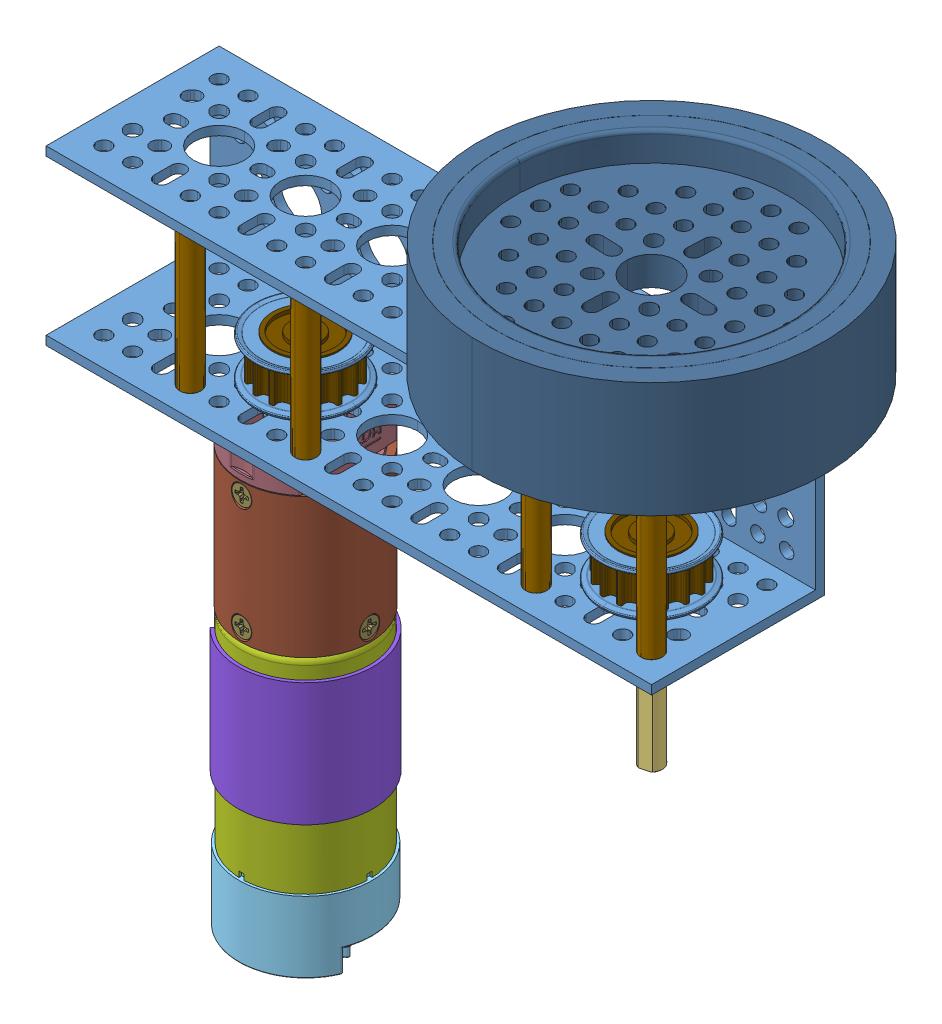
SolidWorks assembly motorisationDroite, configuration Défaut. Lengths in mm.
Overall size (193.77 212.25 99.53).
69 component instances, 28 part files, 30 mates.
Components (placement in the parent):
- 1120-0006-0168 channel-1: 1120-0006-0168 channel [Défaut] at (77.0358 3.4821 146.5) x (0 -1 0) z (0 0 -1) size (48 168 48)
- 5202-2402-0051 moteur-1: 5202-2402-0051 moteur [Défaut] at (-54.0426 -130.9533 205.1707) x (0 0 1) z (-1 0 0) size (52.36 150.75 52.36)
  - 5202-2402-0051.step-1: 5202-2402-0051.step [Défaut] at origin size (52.36 150.75 52.36)
    - 5000-0002-0001.step-1: 5000-0002-0001.step [Défaut] at origin size (52.36 88.75 52.36)
      - 5000-0002-0001 encoder cap.step-1: 5000-0002-0001 encoder cap.step [Défaut] x (0 1 0) z (0 0 1) size (22.84 52.33 52.33)
        - JST-XH-4POS-VERT (1).step-1: JST-XH-4POS-VERT (1).step [Défaut] at (2.8 12.25 -75.95) x (1 0 0) z (0 0 -1) size (10.4 12.83 12.83)
          - Plastic (1).step-1: Plastic (1).step [Défaut] at (-6.1146 -33.6358 -52.1967) x (0 0.707107 0.707107) z (-1 0 0) size (12.4 5.75 7)
          - Pin (1).step-1: Pin (1).step [Défaut] at (-7.7146 -29.3225 -51.2067) x (0 0.707107 0.707107) z (-1 0 0) size (0.64 0.64 10)
          - Pin (1).step-2: Pin (1).step [Défaut] at (-7.7146 -34.6258 -56.51) x (0 0.707107 0.707107) z (-1 0 0) size (0.64 0.64 10)
          - Pin (1).step-3: Pin (1).step [Défaut] at (-7.7146 -32.858 -54.7423) x (0 0.707107 0.707107) z (-1 0 0) size (0.64 0.64 10)
          - Pin (1).step-4: Pin (1).step [Défaut] at (-7.7146 -31.0902 -52.9745) x (0 0.707107 0.707107) z (-1 0 0) size (0.64 0.64 10)
        - screw.step-1: screw.step [Défaut] at (-41.264 -8.1646 3.9905) x (0.882398 0 0.470504) z (0 -1 0) size (8.86 7.85 4.95)
          - 99461A915_Phillips Rounded Head Thread-Forming Screws (1).step-1: 99461A915_Phillips Rounded Head Thread-Forming Screws (1).step [Défaut] at (27.264 -14.6475 -49.347) x (-0.332697 -0.623949 0.707107) z (-0.882398 0.470504 0) size (3.5 3.5 7.4)
        - screw_1.step-1: screw_1.step [Défaut] at (-14.4172 7.3354 3.9905) x (0.882398 0 0.470504) z (0 -1 0) size (8.86 7.85 4.95)
          - 99461A915_Phillips Rounded Head Thread-Forming Screws (1).step-1: 99461A915_Phillips Rounded Head Thread-Forming Screws (1).step [Défaut] at (-10.5142 -28.4382 -25.8237) x (-0.332697 -0.623949 0.707107) z (-0.882398 0.470504 0) size (3.5 3.5 7.4)
        - endcap.step-1: endcap.step [Défaut] at (72.6354 37.1707 -11.0784) x (0 -0.707107 -0.707107) z (1 0 0) size (37 37 21.84)
        - base.step-1: base.step [Défaut] at (-55.8646 37.1707 -11.0784) x (0 -0.707107 -0.707107) z (-1 0 0) size (34.96 34.31 1)
      - 5000-0002-0001 body.step-1: 5000-0002-0001 body.step [Défaut] at (-37.1707 3.4854 -11.0784) size (35.61 61.8 35.61)
      - 5000-0002-0001 motor shield.step-1: 5000-0002-0001 motor shield.step [Défaut] at (-37.1707 54.6354 -11.0784) x (0.808104 0 -0.58904) z (0 -1 0) size (37.5 37.27 34.15)
      - 5000-0002-0001 motor shaft.step-1: 5000-0002-0001 motor shaft.step [Défaut] at (-37.1707 59.4854 -11.0784) size (3.14 12.45 3.14)
    - 5102-0024-0051.step-1: 5102-0024-0051.step [Défaut] at origin size (36 76.68 35.98)
      - 5102 Gearbox Base.step-1: 5102 Gearbox Base.step [Défaut] at (-37.1707 60.1354 -11.0784) size (31.91 5.69 31.91)
      - 5102 Gearbox Barrel (3 stage, simple)_Gear Blank.step-1: 5102 Gearbox Barrel (3 stage, simple)_Gear Blank.step [Défaut] at (-37.1707 111.8354 -11.0784) x (1 0 0) z (0 -1 0) size (35.98 35.98 38.7)
      - 5102 Gearbox Barrel Screw (M3 x 8mm length Flat Head)_92010A118.step-1: 5102 Gearbox Barrel Screw (M3 x 8mm length Flat Head)_92010A118.step [Défaut] at (-37.1707 63.6354 5.0046) x (0.002439 -0.999997 0) z (0 0 1) size (5.46 5.46 8)
      - 5102 Gearbox Face.step-1: 5102 Gearbox Face.step [Défaut] at (-37.1707 93.3354 -11.0784) size (36 17.1 31.91)
      - 5102 Gearbox Bearing.step-1: 5102 Gearbox Bearing.step [Défaut] at (-37.1707 101.4354 -11.0784) size (17 5 17)
      - 5102 Gearbox Shaft (23.5mm Length, Simple).step-1: 5102 Gearbox Shaft (23.5mm Length, Simple).step [Défaut] at (-37.1707 89.9754 -11.0784) x (0.894773 0 -0.44652) z (0.44652 0 0.894773) size (8.97 40.6 8.97)
      - 5102 Gearbox Snap Ring.step-1: 5102 Gearbox Snap Ring.step [Défaut] at (-37.1707 106.5104 -11.0784) x (0 1 0) z (0 0 1) size (0.85 13.06 10.66)
      - 5102 Gearbox Barrel Screw (M3 x 8mm length Flat Head)_92010A118.step-2: 5102 Gearbox Barrel Screw (M3 x 8mm length Flat Head)_92010A118.step [Défaut] at (-37.1707 95.3354 5.0046) x (-0.002439 -0.999997 0) z (0 0 1) size (5.46 5.46 8)
      - 5102 Gearbox Barrel Screw (M3 x 8mm length Flat Head)_92010A118.step-3: 5102 Gearbox Barrel Screw (M3 x 8mm length Flat Head)_92010A118.step [Défaut] at (-21.0877 63.6354 -11.0784) x (0 -0.999997 -0.002439) z (1 0 0) size (5.46 5.46 8)
      - 5102 Gearbox Barrel Screw (M3 x 8mm length Flat Head)_92010A118.step-4: 5102 Gearbox Barrel Screw (M3 x 8mm length Flat Head)_92010A118.step [Défaut] at (-37.1707 63.6354 -27.1614) x (-0.002439 -0.999997 0) z (0 0 -1) size (5.46 5.46 8)
      - 5102 Gearbox Barrel Screw (M3 x 8mm length Flat Head)_92010A118.step-5: 5102 Gearbox Barrel Screw (M3 x 8mm length Flat Head)_92010A118.step [Défaut] at (-53.2537 63.6354 -11.0784) x (0 -0.999997 0.002439) z (-1 0 0) size (5.46 5.46 8)
      - 5102 Gearbox Barrel Screw (M3 x 8mm length Flat Head)_92010A118.step-6: 5102 Gearbox Barrel Screw (M3 x 8mm length Flat Head)_92010A118.step [Défaut] at (-21.0877 95.3354 -11.0784) x (0 -0.999997 0.002439) z (1 0 0) size (5.46 5.46 8)
      - 5102 Gearbox Barrel Screw (M3 x 8mm length Flat Head)_92010A118.step-7: 5102 Gearbox Barrel Screw (M3 x 8mm length Flat Head)_92010A118.step [Défaut] at (-37.1707 95.3354 -27.1614) x (0.002439 -0.999997 0) z (0 0 -1) size (5.46 5.46 8)
      - 5102 Gearbox Barrel Screw (M3 x 8mm length Flat Head)_92010A118.step-8: 5102 Gearbox Barrel Screw (M3 x 8mm length Flat Head)_92010A118.step [Défaut] at (-53.2537 95.3354 -11.0784) x (0 -0.999997 -0.002439) z (-1 0 0) size (5.46 5.46 8)
      - 5102 Gearbox Bearing.step-2: 5102 Gearbox Bearing.step [Défaut] at (-37.1707 93.3354 -11.0784) size (17 5 17)
      - 5102 Gearbox Base Mounting Screw M3 x 5mm length SHCS)_91290A110.step-1: 5102 Gearbox Base Mounting Screw M3 x 5mm length SHCS)_91290A110.step [Défaut] at (-46.0096 57.2554 -2.2396) x (0.056382 0 0.998409) z (0 -1 0) size (5.5 5.5 8)
      - 5102 Gearbox Base Mounting Screw M3 x 5mm length SHCS)_91290A110.step-2: 5102 Gearbox Base Mounting Screw M3 x 5mm length SHCS)_91290A110.step [Défaut] at (-28.3319 57.2554 -2.2396) x (0.998409 0 -0.056382) z (0 -1 0) size (5.5 5.5 8)
      - 5102 Gearbox Base Mounting Screw M3 x 5mm length SHCS)_91290A110.step-3: 5102 Gearbox Base Mounting Screw M3 x 5mm length SHCS)_91290A110.step [Défaut] at (-28.3319 57.2554 -19.9173) x (-0.056382 0 -0.998409) z (0 -1 0) size (5.5 5.5 8)
      - 5102 Gearbox Base Mounting Screw M3 x 5mm length SHCS)_91290A110.step-4: 5102 Gearbox Base Mounting Screw M3 x 5mm length SHCS)_91290A110.step [Défaut] at (-46.0096 57.2554 -19.9173) x (-0.998409 0 0.056382) z (0 -1 0) size (5.5 5.5 8)
- 3417-1006-0016 assembly pulley-1: 3417-1006-0016 assembly pulley [Défaut] at (-65.9677 44.45 158.6429) x (0 1 0) z (1 0 0) size (12.01 27.98 27.98)
  - 3417-1006-0016 assembly.STEP-1: 3417-1006-0016 assembly.STEP [Défaut] at origin size (12.01 27.98 27.98)
    - 3417-1006-0016 body.STEP-1: 3417-1006-0016 body.STEP [Défaut] at (-62.7232 -4.1348 4.7756) size (12 23.97 23.97)
    - 3417-1006-0016 ring.STEP-1: 3417-1006-0016 ring.STEP [Défaut] at (-50.8429 9.3571 23.0035) x (0 -1 0) z (0 0 1) size (27.98 1.38 27.98)
    - 3417-1006-0016 ring.STEP-2: 3417-1006-0016 ring.STEP [Défaut] at (-60.0929 9.3571 23.0035) x (0 -1 0) z (0 0 -1) size (27.98 1.38 27.98)
    - 2806-0005-0006_91390A118.STEP-1: 2806-0005-0006_91390A118.STEP [Défaut] at (-55.4679 9.3571 17.1119) x (-0.607877 0.794031 0) z (0 0 -1) size (5.01 5.01 6.01)
- 3417-1006-0016 assembly pulley-2: 3417-1006-0016 assembly pulley [Défaut] at (61.6463 44.45 144.7068) x (0 1 0) z (0.032246 0 0.99948) size (12.01 27.98 27.98)
  - 3417-1006-0016 assembly.STEP-1: 3417-1006-0016 assembly.STEP [Défaut] at origin size (12.01 27.98 27.98)
    - 3417-1006-0016 body.STEP-1: 3417-1006-0016 body.STEP [Défaut] at (-62.7232 -4.1348 4.7756) size (12 23.97 23.97)
    - 3417-1006-0016 ring.STEP-1: 3417-1006-0016 ring.STEP [Défaut] at (-50.8429 9.3571 23.0035) x (0 -1 0) z (0 0 1) size (27.98 1.38 27.98)
    - 3417-1006-0016 ring.STEP-2: 3417-1006-0016 ring.STEP [Défaut] at (-60.0929 9.3571 23.0035) x (0 -1 0) z (0 0 -1) size (27.98 1.38 27.98)
    - 2806-0005-0006_91390A118.STEP-1: 2806-0005-0006_91390A118.STEP [Défaut] at (-55.4679 9.3571 17.1119) x (-0.607877 0.794031 0) z (0 0 -1) size (5.01 5.01 6.01)
- 2101-0006-0100 essieuCourt-1: 2101-0006-0100 essieuCourt [Défaut] at (53.0358 -61.0179 168) x (-0.964701 0 0.263348) z (-0.263348 0 -0.964701) size (6 100 5.5)
- 1309-0016-1006 assembly-1: 1309-0016-1006 assembly [Défaut] at (69.128 43.7557 176.5253) x (0.868362 0 0.495932) z (0 -1 0) size (28.36 32 10.95)
  - 1309-0016-1006 assembly.STEP-1: 1309-0016-1006 assembly.STEP [Défaut] at origin size (28.36 32 10.95)
    - 1309-0016-1006.STEP-1: 1309-0016-1006.STEP [Défaut] at (-18.2019 0.5776 8.7736) size (25.38 32 10)
    - 2800-0004-0014_90128A207.STEP-1: 2800-0004-0014_90128A207.STEP [Défaut] at (-16.149 11.6963 8.7736) x (0.5 -0.5 -0.707107) z (0.707107 0.707107 0) size (7 7 18.01)
    - 2800-0004-0014_90128A207.STEP-2: 2800-0004-0014_90128A207.STEP [Défaut] at (-20.2547 -10.5411 8.7736) x (-0.5 0.5 -0.707107) z (-0.707107 -0.707107 0) size (7 7 18.01)
- 1611-0514-0006-1: 1611-0514-0006 [Défaut] at (53.0358 -22.0179 168) x (0.99842 0 -0.056195) z (0.056195 0 0.99842) size (15 5 15)
- 1611-0514-0006-2: 1611-0514-0006 [Défaut] at (53.0358 28.9821 168) x (-1 0 0) z (0 0 1) size (15 5 15)
- 2910-0919-0006 assembly collet-2: 2910-0919-0006 assembly collet [Défaut] at (39.3361 19.5025 200.5055) x (-0.7789 0 0.627148) z (-0.627148 0 -0.7789) size (19 9.89 19.83)
  - 2910-0919-0006 assembly.STEP-1: 2910-0919-0006 assembly.STEP [Défaut] at origin size (19 9.89 19.83)
    - 2910-0919-0006.STEP-1: 2910-0919-0006.STEP [Défaut] at (-31.0565 -0.5204 16.7268) size (19 9.5 18.97)
    - 2800-0004-0010_90128A207.STEP-1: 2800-0004-0010_90128A207.STEP [Défaut] at (-24.2865 -0.5204 11.2868) x (0 -0.807243 -0.59022) z (1 0 0) size (7 7 14.01)
- 1501-0006-0430 renfort-1: 1501-0006-0430 renfort [Défaut] at (69.0358 3.4821 184) size (5.95 43.01 5.95)
- 1501-0006-0430 renfort-2: 1501-0006-0430 renfort [Défaut] at (37.0358 3.4821 184) size (5.95 43.01 5.95)
- 1501-0006-0430 renfort-3: 1501-0006-0430 renfort [Défaut] at (-58.9642 3.4821 184) size (5.95 43.01 5.95)
- 1501-0006-0430 renfort-4: 1501-0006-0430 renfort [Défaut] at (-26.9642 3.4821 184) size (5.95 43.01 5.95)
- 3601-0014-0096 part-1: 3601-0014-0096 part [Défaut] at (53.0358 32.4821 168) x (-0.999296 0 -0.037515) z (0 -1 0) size (96 96 32)
Mates (geometry in assembly coordinates):
- Coaxiale1: concentric: cylinder of 5202-2402-0051 moteur-1/5202-2402-0051.step-1/5102-0024-0051.step-1/5102 Gearbox Shaft (23.5mm Length, Simple).step-1 through (-42.9642 -22.5179 168) axis (0 1 0) radius 3; cylinder of 1120-0006-0168 channel-1 through (-42.9642 -10.5179 168) axis (0 -1 0) radius 7
- Coïncidente1: coincident: plane of 1120-0006-0168 channel-1 through (-90.9642 -20.5179 192) normal (0 -1 0); plane of 5202-2402-0051 moteur-1/5202-2402-0051.step-1/5102-0024-0051.step-1/5102 Gearbox Face.step-1 through (-42.9642 -20.5179 168) normal (0 1 0)
- Coaxiale7: concentric: cylinder of 5202-2402-0051 moteur-1/5202-2402-0051.step-1/5102-0024-0051.step-1/5102 Gearbox Shaft (23.5mm Length, Simple).step-1 through (-42.9642 -22.5179 168) axis (0 1 0) radius 3; cylinder of 3417-1006-0016 assembly pulley-1/3417-1006-0016 assembly.STEP-1/3417-1006-0016 body.STEP-1 through (-42.9642 -27.648 168) axis (0 1 0) radius 3
- Parallèle2: parallel: plane of 5202-2402-0051 moteur-1/5202-2402-0051.step-1/5102-0024-0051.step-1/5102 Gearbox Shaft (23.5mm Length, Simple).step-1 through (-45.4142 -22.5179 171.7567) normal (-1 0 0); line of 3417-1006-0016 assembly pulley-1/3417-1006-0016 assembly.STEP-1/3417-1006-0016 body.STEP-1 through (-45.4442 -5.0179 166.3119) axis (0 0 1)
- Coaxiale8: concentric: cylinder of 1120-0006-0168 channel-1 through (53.0358 17.4821 168) axis (0 1 0) radius 7; cylinder of 3417-1006-0016 assembly pulley-2/3417-1006-0016 assembly.STEP-1/3417-1006-0016 body.STEP-1 through (53.0358 -27.648 168) axis (0 1 0) radius 3
- Coaxiale10: concentric: cylinder of 1120-0006-0168 channel-1 through (53.0358 -10.5179 168) axis (0 -1 0) radius 7; cylinder of 2101-0006-0100 essieuCourt-1 through (53.0358 38.9821 168) axis (0 -1 0) radius 3
- Coaxiale14: concentric: cylinder of 1120-0006-0168 channel-1 through (53.0358 -10.5179 168) axis (0 -1 0) radius 7; cylinder of 1611-0514-0006-2 through (53.0358 28.9821 168) axis (0 -1 0) radius 3
- Coaxiale15: concentric: cylinder of 2101-0006-0100 essieuCourt-1 through (53.0358 38.9821 168) axis (0 -1 0) radius 3; cylinder of 1611-0514-0006-1 through (53.0358 -22.0179 168) axis (0 1 0) radius 3
- Coïncidente12: coincident: plane of 1120-0006-0168 channel-1 through (-90.9642 24.9821 146.5) normal (0 -1 0); plane of 1611-0514-0006-2 through (53.0358 24.9821 168) normal (0 1 0)
- Coïncidente13: coincident: plane of 1120-0006-0168 channel-1 through (-90.9642 -18.0179 146.5) normal (0 1 0); plane of 1611-0514-0006-1 through (53.0358 -18.0179 168) normal (0 -1 0)
- Parallèle4: parallel: plane of 3417-1006-0016 assembly pulley-2/3417-1006-0016 assembly.STEP-1/3417-1006-0016 body.STEP-1 through (53.0358 -17.0179 168) normal (0 -1 0); plane of 1611-0514-0006-1 through (53.0358 -17.0179 168) normal (0 1 0)
- Coïncidente15: coincident: plane of 3417-1006-0016 assembly pulley-2/3417-1006-0016 assembly.STEP-1/3417-1006-0016 body.STEP-1 through (53.0358 -17.0179 168) normal (0 -1 0); plane of 1611-0514-0006-1 through (53.0358 -17.0179 168) normal (0 1 0)
- Coaxiale17: concentric: cylinder of 1120-0006-0168 channel-1 through (53.0358 -10.5179 168) axis (0 -1 0) radius 7; cylinder of 2910-0919-0006 assembly collet-2/2910-0919-0006 assembly.STEP-1/2910-0919-0006.STEP-1 through (53.0358 23.4821 168) axis (0 -1 0) radius 3
- Coïncidente18: coincident: plane of 1611-0514-0006-2 through (53.0358 23.9821 168) normal (0 -1 0); plane of 2910-0919-0006 assembly collet-2/2910-0919-0006 assembly.STEP-1/2910-0919-0006.STEP-1 through (53.0358 23.9821 168) normal (0 1 0)
- Coïncidente21: coincident: plane of 1120-0006-0168 channel-1 through (-90.9642 -18.0179 146.5) normal (0 1 0); plane of 1501-0006-0430 renfort-1 through (69.0358 -18.0179 184) normal (0 -1 0)
- Coïncidente22: coincident: plane of 1120-0006-0168 channel-1 through (-90.9642 -18.0179 146.5) normal (0 1 0); plane of 1501-0006-0430 renfort-2 through (37.0358 -18.0179 184) normal (0 -1 0)
- Coaxiale18: concentric: cylinder of 1120-0006-0168 channel-1 through (69.0358 -10.5179 184) axis (0 -1 0) radius 2; cylinder of 1501-0006-0430 renfort-1 through (69.0358 24.9821 184) axis (0 -1 0) radius 2.975
- Coaxiale19: concentric: circle of 1120-0006-0168 channel-1; cylinder of 1501-0006-0430 renfort-2 through (37.0358 24.9821 184) axis (0 -1 0) radius 2.975
- Coïncidente23: coincident: plane of 3417-1006-0016 assembly pulley-1/3417-1006-0016 assembly.STEP-1/3417-1006-0016 body.STEP-1 through (-36.6423 -5.0179 177.8863) normal (0 1 0); plane of 3417-1006-0016 assembly pulley-2/3417-1006-0016 assembly.STEP-1/3417-1006-0016 body.STEP-1 through (43.3585 -5.0179 174.6374) normal (0 1 0)
- Coïncidente24: coincident: plane of 1120-0006-0168 channel-1 through (-90.9642 -18.0179 146.5) normal (0 1 0); plane of 1501-0006-0430 renfort-4 through (-26.9642 -18.0179 184) normal (0 -1 0)
- Coïncidente25: coincident: plane of 1120-0006-0168 channel-1 through (-90.9642 -18.0179 146.5) normal (0 1 0); plane of 1501-0006-0430 renfort-3 through (-82.9642 -18.0179 184) normal (0 -1 0)
- Coaxiale20: concentric: cylinder of 1501-0006-0430 renfort-3 through (-58.9642 24.9821 184) axis (0 -1 0) radius 2.975; cylinder of 1120-0006-0168 channel-1 through (-58.9642 -10.5179 184) axis (0 -1 0) radius 2
- Coaxiale21: concentric: cylinder of 1501-0006-0430 renfort-4 through (-26.9642 24.9821 184) axis (0 -1 0) radius 2.975; cylinder of 1120-0006-0168 channel-1 through (-26.9642 -10.5179 184) axis (0 -1 0) radius 2
- Coaxiale22: concentric: cylinder of 2101-0006-0100 essieuCourt-1 through (53.0358 38.9821 168) axis (0 -1 0) radius 3; cylinder of 3601-0014-0096 part-1 through (53.0358 32.4821 168) axis (0 1 0) radius 7
- Distance1: distance = 5 mm: plane of 3601-0014-0096 part-1 through (53.0358 32.4821 168) normal (0 -1 0); plane of 1120-0006-0168 channel-1 through (-90.9642 27.4821 192) normal (0 1 0)
- Parallèle5: parallel: plane of 2101-0006-0100 essieuCourt-1 through (53.6942 38.9821 170.4118) normal (0.263348 0 0.964701); plane of 1309-0016-1006 assembly-1/1309-0016-1006 assembly.STEP-1/1309-0016-1006.STEP-1 through (53.6889 39.2326 170.3925) normal (-0.263348 0 -0.964701)
- Coaxiale23: concentric: cylinder of 2101-0006-0100 essieuCourt-1 through (53.0358 38.9821 168) axis (0 -1 0) radius 3; cylinder of 1309-0016-1006 assembly-1/1309-0016-1006 assembly.STEP-1/1309-0016-1006.STEP-1 through (53.0358 39.2326 168) axis (0 -1 0) radius 3
- Coïncidente27: coincident: plane of 1309-0016-1006 assembly-1/1309-0016-1006 assembly.STEP-1/1309-0016-1006.STEP-1 through (53.0358 28.9821 168) normal (0 -1 0); plane of 1611-0514-0006-2 through (53.0358 28.9821 168) normal (0 1 0)
- Coïncidente28: coincident: plane of 2101-0006-0100 essieuCourt-1 through (53.0358 38.9821 168) normal (0 1 0); plane of 1309-0016-1006 assembly-1/1309-0016-1006 assembly.STEP-1/1309-0016-1006.STEP-1 through (53.0358 38.9821 168) normal (0 1 0)
- Coaxiale24: concentric: circle of 1120-0006-0168 channel-1; circle of 5202-2402-0051 moteur-1/5202-2402-0051.step-1/5102-0024-0051.step-1/5102 Gearbox Face.step-1
